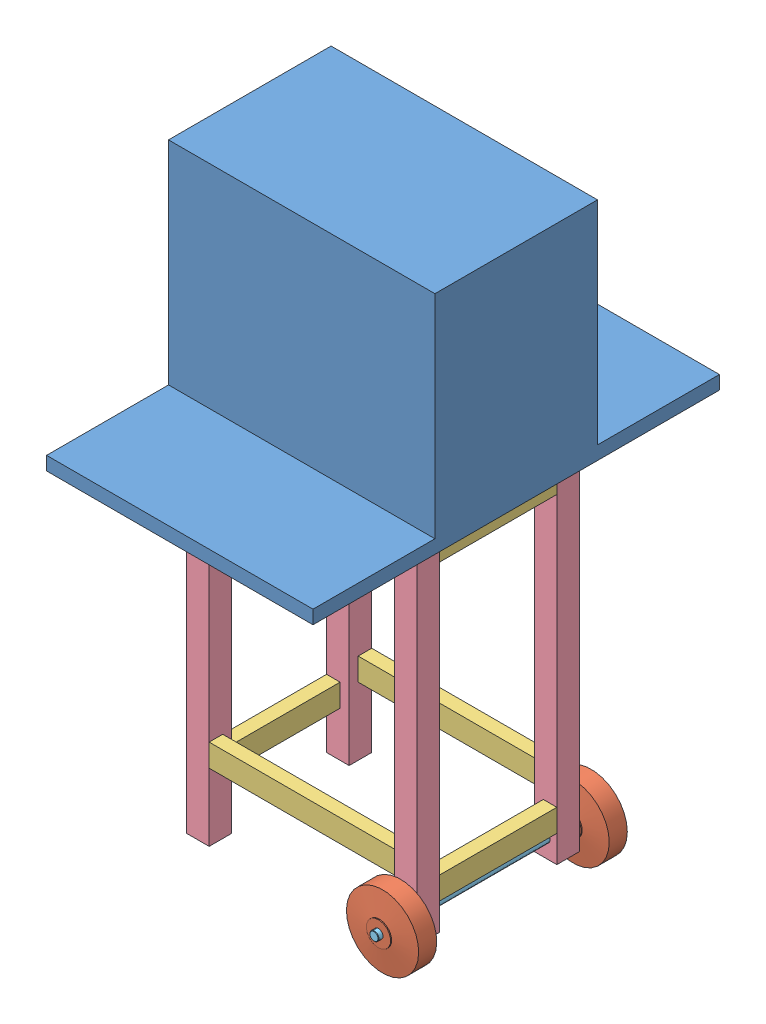
SolidWorks assembly ps_assy, configuration Default. Lengths in mm.
Overall size (621.47 1326.47 900).
17 component instances, 6 part files, 43 mates.
Components (placement in the parent):
- ps_metabo_planer-1: ps_metabo_planer [Default] at (-330.6347 810 -145.4799) size (590 510 900)
- ps_wheel_160-1: ps_wheel_160 [Default] at (194.3653 80 245.5201) x (0 0 1) z (-0.97237 0.233445 0) size (58 160 160)
- ps_wheel_160-2: ps_wheel_160 [Default] at (194.3653 80 -176.4799) x (0 0 -1) z (1 0 0) size (58 160 160)
- ps_frame_pt1-1: ps_frame_pt1 [front] at (-240.6347 750 214.5201) x (0 0 -1) z (1 0 0) size (30 50 410)
- ps_frame_pt1-2: ps_frame_pt1 [front] at (-240.6347 750 -115.4799) x (0 0 -1) z (1 0 0) size (30 50 410)
- ps_frame_pt1-3: ps_frame_pt1 [side] at (-290.6347 700 -95.4799) size (30 50 260)
- ps_frame_pt1-4: ps_frame_pt1 [side] at (189.3653 750 -95.4799) size (30 50 260)
- ps_frame_pt2-1: ps_frame_pt2 [Front] at (-290.6347 0 -95.4799) size (50 800 50)
- ps_frame_pt2-2: ps_frame_pt2 [Front] at (-290.6347 0 214.5201) size (50 800 50)
- ps_frame_pt2-3: ps_frame_pt2 [Back] at (169.3653 40 -95.4799) size (50 760 50)
- ps_frame_pt2-4: ps_frame_pt2 [Back] at (169.3653 40 214.5201) size (50 760 50)
- ps_frame_pt1-5: ps_frame_pt1 [side] at (189.3653 100 -95.4799) size (30 50 260)
- ps_frame_pt1-6: ps_frame_pt1 [side] at (-290.6347 100 -95.4799) size (30 50 260)
- ps_frame_pt1-7: ps_frame_pt1 [front] at (-240.6347 150 214.5201) x (0 0 -1) z (1 0 0) size (30 50 410)
- ps_round_bar_20mm-1: ps_round_bar_20mm [Default] at (194.3653 80 -215.4799) size (20 20 500)
- ps_frame_pt1-8: ps_frame_pt1 [front] at (-240.6347 150 -115.4799) x (0 0 -1) z (1 0 0) size (30 50 410)
- Mitre Saw -  Large Assembly-1: Mitre Saw -  Large Assembly [Default] at (-42.3222 808.431 25.8674) size (696.28 633.81 985.62) (hidden)
Mates (geometry in assembly coordinates):
- Coïncidente10: coincident anti-aligned: plane of ps_frame_pt1-3 through (-290.6347 700 -95.4799) normal (0 0 -1); plane of ps_frame_pt2-1 through (-290.6347 800 -95.4799) normal (0 0 1)
- Coïncidente11: coincident aligned: plane of ps_frame_pt1-3 through (-290.6347 700 164.5201) normal (-1 0 0); plane of ps_frame_pt2-1 through (-290.6347 800 -95.4799) normal (-1 0 0)
- Coïncidente13: coincident anti-aligned: plane of ps_frame_pt1-2 through (-240.6347 750 -115.4799) normal (-1 0 0); plane of ps_frame_pt2-1 through (-240.6347 800 -95.4799) normal (1 0 0)
- Coïncidente14: coincident aligned: plane of ps_frame_pt1-2 through (169.3653 750 -145.4799) normal (0 0 -1); plane of ps_frame_pt2-1 through (-290.6347 800 -145.4799) normal (0 0 -1)
- Coïncidente16: coincident anti-aligned: plane of ps_frame_pt1-3 through (-290.6347 700 164.5201) normal (0 0 1); plane of ps_frame_pt2-2 through (-290.6347 800 164.5201) normal (0 0 -1)
- Coïncidente17: coincident aligned: plane of ps_frame_pt1-3 through (-290.6347 700 164.5201) normal (-1 0 0); plane of ps_frame_pt2-2 through (-290.6347 800 214.5201) normal (-1 0 0)
- Coïncidente19: coincident anti-aligned: plane of ps_frame_pt1-1 through (-240.6347 750 214.5201) normal (-1 0 0); plane of ps_frame_pt2-2 through (-240.6347 800 214.5201) normal (1 0 0)
- Coïncidente20: coincident aligned: plane of ps_frame_pt1-1 through (169.3653 750 214.5201) normal (0 0 1); plane of ps_frame_pt2-2 through (-290.6347 800 214.5201) normal (0 0 1)
- Coïncidente22: coincident anti-aligned: plane of ps_frame_pt1-1 through (169.3653 750 214.5201) normal (1 0 0); plane of ps_frame_pt2-4 through (169.3653 800 214.5201) normal (-1 0 0)
- Coïncidente25: coincident aligned: plane of ps_frame_pt1-1 through (169.3653 750 214.5201) normal (0 0 1); plane of ps_frame_pt2-4 through (169.3653 800 214.5201) normal (0 0 1)
- Coïncidente26: coincident anti-aligned: plane of ps_frame_pt1-4 through (189.3653 750 164.5201) normal (0 0 1); plane of ps_frame_pt2-4 through (169.3653 800 164.5201) normal (0 0 -1)
- Coïncidente27: coincident aligned: plane of ps_frame_pt1-4 through (219.3653 750 164.5201) normal (1 0 0); plane of ps_frame_pt2-4 through (219.3653 800 214.5201) normal (1 0 0)
- Coïncidente28: coincident anti-aligned: plane of ps_frame_pt1-4 through (189.3653 750 -95.4799) normal (0 0 -1); plane of ps_frame_pt2-3 through (169.3653 800 -95.4799) normal (0 0 1)
- Coïncidente29: coincident aligned: plane of ps_frame_pt1-4 through (189.3653 800 164.5201) normal (0 1 0); plane of ps_frame_pt2-3 through (169.3653 800 -95.4799) normal (0 1 0)
- Coïncidente30: coincident aligned: plane of ps_frame_pt1-4 through (219.3653 750 164.5201) normal (1 0 0); plane of ps_frame_pt2-3 through (219.3653 800 -95.4799) normal (1 0 0)
- Coïncidente31: coincident anti-aligned: plane of ps_frame_pt2-4 through (169.3653 800 164.5201) normal (0 0 -1); plane of ps_frame_pt1-5 through (189.3653 100 164.5201) normal (0 0 1)
- Coïncidente32: coincident aligned: plane of ps_frame_pt2-4 through (219.3653 800 214.5201) normal (1 0 0); plane of ps_frame_pt1-5 through (219.3653 100 164.5201) normal (1 0 0)
- Coïncidente33: coincident anti-aligned: plane of ps_frame_pt2-2 through (-290.6347 800 164.5201) normal (0 0 -1); plane of ps_frame_pt1-6 through (-290.6347 100 164.5201) normal (0 0 1)
- Coïncidente34: coincident aligned: plane of ps_frame_pt2-2 through (-290.6347 800 214.5201) normal (-1 0 0); plane of ps_frame_pt1-6 through (-290.6347 100 164.5201) normal (-1 0 0)
- Coïncidente35: coincident aligned: plane of ps_frame_pt1-5 through (189.3653 150 164.5201) normal (0 1 0); plane of ps_frame_pt1-6 through (-290.6347 150 164.5201) normal (0 1 0)
- Coïncidente37: coincident anti-aligned: plane of ps_frame_pt2-4 through (169.3653 800 214.5201) normal (-1 0 0); plane of ps_frame_pt1-7 through (169.3653 150 214.5201) normal (1 0 0)
- Coïncidente38: coincident aligned: plane of ps_frame_pt2-4 through (169.3653 800 214.5201) normal (0 0 1); plane of ps_frame_pt1-7 through (169.3653 150 214.5201) normal (0 0 1)
- Coïncidente39: coincident anti-aligned: plane of ps_metabo_planer-1 through (-330.6347 800 -145.4799) normal (0 -1 0); plane of ps_frame_pt2-2 through (-290.6347 800 214.5201) normal (0 1 0)
- Coïncidente40: coincident aligned: plane of ps_frame_pt1-1 through (169.3653 800 214.5201) normal (0 1 0); plane of ps_frame_pt1-2 through (169.3653 800 -115.4799) normal (0 1 0)
- Coaxiale1: concentric anti-aligned: cylinder of ps_wheel_160-1 through (194.3653 80 245.5201) axis (0 0 -1) radius 80; cylinder of ps_wheel_160-2 through (194.3653 80 -176.4799) axis (0 0 1) radius 80
- Coaxiale2: concentric anti-aligned: cylinder of ps_wheel_160-1 through (194.3653 80 245.5201) axis (0 0 -1) radius 10; cylinder of ps_frame_pt2-3 through (194.3653 80 -145.4799) axis (0 0 1) radius 10
- Distance1: distance = 2 mm anti-aligned: plane of ps_wheel_160-1 through (200.6683 106.254 216.5201) normal (0 0 -1); plane of ps_frame_pt2-4 through (169.3653 800 214.5201) normal (0 0 1)
- Distance2: distance = 2 mm anti-aligned: plane of ps_wheel_160-2 through (194.3653 107 -147.4799) normal (0 0 1); plane of ps_frame_pt2-3 through (169.3653 800 -145.4799) normal (0 0 -1)
- Coaxiale3: concentric anti-aligned: cylinder of ps_wheel_160-1 through (194.3653 80 245.5201) axis (0 0 -1) radius 10; cylinder of ps_frame_pt2-4 through (194.3653 80 164.5201) axis (0 0 1) radius 10
- Coïncidente43: coincident anti-aligned: plane of ps_metabo_planer-1 through (-330.6347 800 -145.4799) normal (0 -1 0); plane of ps_frame_pt2-4 through (169.3653 800 214.5201) normal (0 1 0)
- Coïncidente45: coincident anti-aligned: plane of ps_frame_pt1-5 through (189.3653 150 164.5201) normal (0 1 0); plane of ps_frame_pt1-7 through (169.3653 150 214.5201) normal (0 -1 0)
- Distance3: distance = 60 mm aligned: plane of ps_frame_pt1-5 through (189.3653 100 164.5201) normal (0 -1 0); plane of ps_frame_pt2-3 through (169.3653 40 -95.4799) normal (0 -1 0)
- Coïncidente46: coincident aligned: plane of ps_metabo_planer-1 through (-330.6347 810 214.5201) normal (0 0 1); plane of ps_frame_pt2-4 through (169.3653 800 214.5201) normal (0 0 1)
- Distance4: distance = 10 mm aligned: plane of ps_frame_pt2-4 through (219.3653 800 214.5201) normal (1 0 0); plane of ps_metabo_planer-1 through (229.3653 800 -145.4799) normal (1 0 0)
- Coïncidente47: coincident aligned: plane of ps_frame_pt1-1 through (169.3653 800 214.5201) normal (0 1 0); plane of ps_frame_pt2-2 through (-290.6347 800 214.5201) normal (0 1 0)
- Coïncidente48: coincident anti-aligned: plane of ps_frame_pt1-1 through (169.3653 750 214.5201) normal (0 -1 0); plane of ps_frame_pt1-3 through (-290.6347 750 164.5201) normal (0 1 0)
- Coaxiale4: concentric aligned: cylinder of ps_wheel_160-1 through (194.3653 80 245.5201) axis (0 0 -1) radius 10; cylinder of ps_round_bar_20mm-1 through (194.3653 80 284.5201) axis (0 0 -1) radius 10
- Distance5: distance = 10 mm aligned: plane of ps_wheel_160-1 through (200.6683 106.254 274.5201) normal (0 0 1); plane of ps_round_bar_20mm-1 through (194.3653 80 284.5201) normal (0 0 1)
- Coïncidente50: coincident anti-aligned: plane of ps_metabo_planer-1 through (-330.6347 800 -145.4799) normal (0 -1 0); plane of ps_frame_pt2-1 through (-290.6347 800 -95.4799) normal (0 1 0)
- Coïncidente51: coincident anti-aligned: plane of ps_frame_pt2-1 through (-240.6347 800 -95.4799) normal (1 0 0); plane of ps_frame_pt1-8 through (-240.6347 150 -115.4799) normal (-1 0 0)
- Coïncidente52: coincident aligned: plane of ps_frame_pt2-1 through (-290.6347 800 -145.4799) normal (0 0 -1); plane of ps_frame_pt1-8 through (169.3653 150 -145.4799) normal (0 0 -1)
- Coïncidente53: coincident aligned: plane of ps_frame_pt1-7 through (169.3653 200 214.5201) normal (0 1 0); plane of ps_frame_pt1-8 through (169.3653 200 -115.4799) normal (0 1 0)
- Coïncidente54: coincident anti-aligned: plane of ps_frame_pt2-2 through (-290.6347 0 214.5201) normal (0 -1 0); plane of assembly through (0 0 0) normal (0 1 0)
